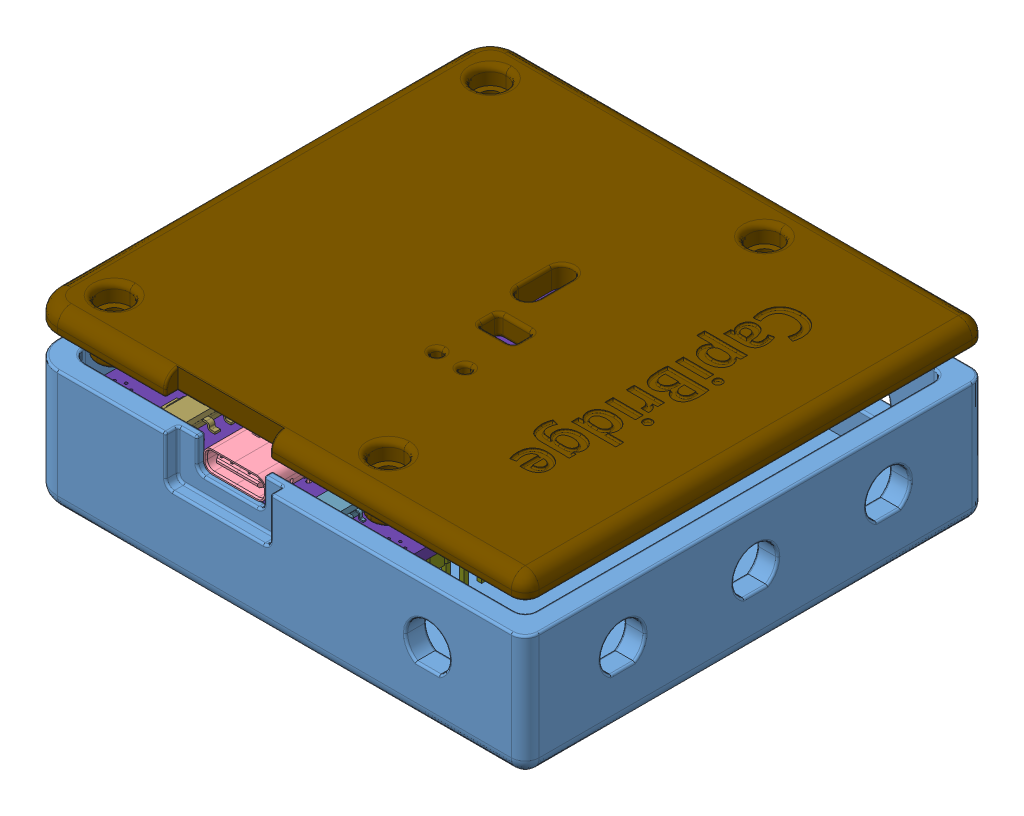
SolidWorks assembly Assem1, configuration Default. Lengths in mm.
Overall size (71 24.85 66.01).
68 component instances, 18 part files, 4 mates.
Components (placement in the parent):
- CapiBridge_Case.step-1: CapiBridge_Case.step [Default] at (49.0478 21.2808 49.0747) size (71 17.5 66.01)
- CapiBridge_PCB.step-1: CapiBridge_PCB.step [Default] at (23.5288 30.2808 76.9234) x (1 0 0) z (0 1 0) size (44.35 60.13 16.04)
  - C_0603_1608Metric.step-1: C_0603_1608Metric.step [Default] at (19.4987 21.1736 1.65) x (0 1 0) z (0 0 1) size (1.6 0.8 0.8)
    - C_0603_1608Metric-0.step-1: C_0603_1608Metric-0.step [Default] at origin size (1.6 0.8 0.8)
  - CP_EIA-3216-18_Kemet-A.step-1: CP_EIA-3216-18_Kemet-A.step [Default] at (11.2987 11.0736 1.65) size (3.2 1.6 1.8)
    - CP_EIA_3216_18_Kemet_A.step-1: CP_EIA_3216_18_Kemet_A.step [Default] at origin size (3.2 1.6 1.8)
  - USB_C_Receptacle_GCT_USB4105-xx-A_16P_TopMnt_Horizontal.step-1: USB_C_Receptacle_GCT_USB4105-xx-A_16P_TopMnt_Horizontal.step [Default] at (17.0087 0.9136 1.65) size (8.94 7.78 4.26)
    - USB_C_Receptacle_16P_TopMnt_Horizontal_GCT_USB4105-xx-A.step-1: USB_C_Receptacle_16P_TopMnt_Horizontal_GCT_USB4105-xx-A.step [Default] at origin size (8.94 7.78 4.26)
  - LED_0603_1608Metric.step-1: LED_0603_1608Metric.step [Default] at (25.3487 32.6736 1.65) size (1.6 0.8 1.1)
    - LED_0603_1608Metric-1.step-1: LED_0603_1608Metric-1.step [Default] at origin size (1.6 0.8 1.1)
  - YC164-FR-075K6L.step-1: YC164-FR-075K6L.step [Default] at (30.4987 33.3236 1.65) x (1 0 0) z (0 -1 0) size (1.6 0.7 3.2)
    - YC164-JR-0720KL.step-1: YC164-JR-0720KL.step [Default] at origin size (1.6 0.7 3.2)
  - CP_EIA-3528-21_Kemet-B.step-1: CP_EIA-3528-21_Kemet-B.step [Default] at (1.7987 9.5736 1.65) x (0 1 0) z (0 0 1) size (3.5 2.8 2.1)
    - CP_EIA_3528_21_Kemet_B.step-1: CP_EIA_3528_21_Kemet_B.step [Default] at origin size (3.5 2.8 2.1)
  - LED_0603_1608Metric.step-2: LED_0603_1608Metric.step [Default] at (25.3487 34.2236 1.65) size (1.6 0.8 1.1)
    - LED_0603_1608Metric-1.step-1: LED_0603_1608Metric-1.step [Default] at origin size (1.6 0.8 1.1)
  - ESP32-C3-WROOM-02U-N4.step-1: ESP32-C3-WROOM-02U-N4.step [Default] at (15.9527 35.9396 1.65) size (18 14.3 3.21)
    - 3D_PCB1_2022-06-18 v3.step-1: 3D_PCB1_2022-06-18 v3.step [Default] at origin size (18 14.3 3.21)
  - YC164-FR-075K6L.step-2: YC164-FR-075K6L.step [Default] at (20.3487 26.0736 1.65) x (0 -1 0) z (-1 0 0) size (1.6 0.7 3.2)
    - YC164-JR-0720KL.step-1: YC164-JR-0720KL.step [Default] at origin size (1.6 0.7 3.2)
  - C_0603_1608Metric.step-2: C_0603_1608Metric.step [Default] at (32.0987 6.8736 1.65) x (0 -1 0) z (0 0 1) size (1.6 0.8 0.8)
    - C_0603_1608Metric-0.step-1: C_0603_1608Metric-0.step [Default] at origin size (1.6 0.8 0.8)
  - SOT-363_SC-70-6.step-1: SOT-363_SC-70-6.step [Default] at (26.2487 11.2236 1.65) x (-1 0 0) z (0 0 1) size (2 2 1.05)
    - SOT_363_SC_70_6.step-1: SOT_363_SC_70_6.step [Default] at origin size (2 2 1.05)
  - RA-01H--3DModel-STEP-1.step-1: RA-01H--3DModel-STEP-1.step [Default] at (8.3787 22.6736 1.65) x (1 0 0) z (0 -1 0) size (16 3.4 17)
    - RA-01H.step-1: RA-01H.step [Default] at origin size (16 3.4 17)
  - C_0603_1608Metric.step-3: C_0603_1608Metric.step [Default] at (-1.8853 26.4736 1.65) x (0 1 0) z (0 0 1) size (1.6 0.8 0.8)
    - C_0603_1608Metric-0.step-1: C_0603_1608Metric-0.step [Default] at origin size (1.6 0.8 0.8)
  - SOT-143.step-1: SOT-143.step [Default] at (16.9851 8.7089 1.65) size (2.8 2.9 1.2)
    - SOT_143.step-1: SOT_143.step [Default] at origin size (2.8 2.9 1.2)
  - C_0603_1608Metric.step-4: C_0603_1608Metric.step [Default] at (-5.1336 49.1028 1.65) x (0 -1 0) z (0 0 1) size (1.6 0.8 0.8)
    - C_0603_1608Metric-0.step-1: C_0603_1608Metric-0.step [Default] at origin size (1.6 0.8 0.8)
  - C_0603_1608Metric.step-5: C_0603_1608Metric.step [Default] at (4.4987 9.0736 1.65) x (0 1 0) z (0 0 1) size (1.6 0.8 0.8)
    - C_0603_1608Metric-0.step-1: C_0603_1608Metric-0.step [Default] at origin size (1.6 0.8 0.8)
  - ESP32-C3-WROOM-02U-N4.step-2: ESP32-C3-WROOM-02U-N4.step [Default] at (-5.1973 35.9656 1.65) size (18 14.3 3.21)
    - 3D_PCB1_2022-06-18 v3.step-1: 3D_PCB1_2022-06-18 v3.step [Default] at origin size (18 14.3 3.21)
  - SOT-223.step-1: SOT-223.step [Default] at (5.3487 2.9736 1.65) x (-1 0 0) z (0 0 1) size (7 6.5 1.7)
    - SOT_223.step-1: SOT_223.step [Default] at origin size (7 6.5 1.7)
  - YC164-FR-075K6L.step-3: YC164-FR-075K6L.step [Default] at (30.4487 11.6736 1.65) x (1 0 0) z (0 -1 0) size (1.6 0.7 3.2)
    - YC164-JR-0720KL.step-1: YC164-JR-0720KL.step [Default] at origin size (1.6 0.7 3.2)
  - C_0603_1608Metric.step-6: C_0603_1608Metric.step [Default] at (21.0987 21.1736 1.65) x (0 1 0) z (0 0 1) size (1.6 0.8 0.8)
    - C_0603_1608Metric-0.step-1: C_0603_1608Metric-0.step [Default] at origin size (1.6 0.8 0.8)
  - LED_0603_1608Metric.step-3: LED_0603_1608Metric.step [Default] at (25.3487 35.8236 1.65) size (1.6 0.8 1.1)
    - LED_0603_1608Metric-1.step-1: LED_0603_1608Metric-1.step [Default] at origin size (1.6 0.8 1.1)
  - Selector Switch - MSS22D18.step-1: Selector Switch - MSS22D18.step [Default] at (28.2987 27.1236 6.9) x (1 0 0) z (0 -1 0) size (9.17 5.82 6.22)
    - Selector Switch - MSS22D18-2.step-1: Selector Switch - MSS22D18-2.step [Default] at origin size (9.17 5.82 6.22)
  - LED_0603_1608Metric.step-4: LED_0603_1608Metric.step [Default] at (20.4487 10.4236 1.65) x (0 1 0) z (0 0 1) size (1.6 0.8 1.1)
    - LED_0603_1608Metric-1.step-1: LED_0603_1608Metric-1.step [Default] at origin size (1.6 0.8 1.1)
  - SOIC-16_3.9x9.9mm_P1.27mm.step-1: SOIC-16_3.9x9.9mm_P1.27mm.step [Default] at (27.3987 4.3736 1.65) size (6 9.9 1.75)
    - SOIC_16_39x99mm_P127mm.step-1: SOIC_16_39x99mm_P127mm.step [Default] at origin size (6 9.9 1.75)
  - C_0603_1608Metric.step-7: C_0603_1608Metric.step [Default] at (16.0807 49.1515 1.65) x (0 1 0) z (0 0 1) size (1.6 0.8 0.8)
    - C_0603_1608Metric-0.step-1: C_0603_1608Metric-0.step [Default] at origin size (1.6 0.8 0.8)
  - LED_0603_1608Metric.step-5: LED_0603_1608Metric.step [Default] at (22.1487 10.4236 1.65) x (0 1 0) z (0 0 1) size (1.6 0.8 1.1)
    - LED_0603_1608Metric-1.step-1: LED_0603_1608Metric-1.step [Default] at origin size (1.6 0.8 1.1)
  - C_0603_1608Metric.step-8: C_0603_1608Metric.step [Default] at (7.3487 9.8736 1.65) x (-1 0 0) z (0 0 1) size (1.6 0.8 0.8)
    - C_0603_1608Metric-0.step-1: C_0603_1608Metric-0.step [Default] at origin size (1.6 0.8 0.8)
  - LED_0603_1608Metric.step-6: LED_0603_1608Metric.step [Default] at (25.3487 31.0736 1.65) size (1.6 0.8 1.1)
    - LED_0603_1608Metric-1.step-1: LED_0603_1608Metric-1.step [Default] at origin size (1.6 0.8 1.1)
  - D_SOD-123F.step-1: D_SOD-123F.step [Default] at (11.2987 8.6736 1.65) size (3.5 1.6 1.1)
    - D_SOD_123F.step-1: D_SOD_123F.step [Default] at origin size (3.5 1.6 1.1)
  - YC164-FR-075K6L.step-4: YC164-FR-075K6L.step [Default] at (20.2987 16.4736 1.65) x (0 1 0) z (1 0 0) size (1.6 0.7 3.2)
    - YC164-JR-0720KL.step-1: YC164-JR-0720KL.step [Default] at origin size (1.6 0.7 3.2)
  - PinHeader_1x12_P2.54mm_Vertical.step-1: PinHeader_1x12_P2.54mm_Vertical.step [Default] at (-4.62 5.9936 -0.05) x (1 0 0) z (0 0 -1) size (2.54 30.48 11.54)
    - PinHeader_1x12_P254mm_Vertical.step-1: PinHeader_1x12_P254mm_Vertical.step [Default] at origin size (2.54 30.48 11.54)
  - PinHeader_1x12_P2.54mm_Vertical.step-2: PinHeader_1x12_P2.54mm_Vertical.step [Default] at (36.02 5.9736 -0.05) x (1 0 0) z (0 0 -1) size (2.54 30.48 11.54)
    - PinHeader_1x12_P254mm_Vertical.step-1: PinHeader_1x12_P254mm_Vertical.step [Default] at origin size (2.54 30.48 11.54)
  - ESP-NOW_Gateway_PCB.step-1: ESP-NOW_Gateway_PCB.step [Default] at origin size (44.35 58.95 1.6)
- CapiBridge_Case_lit.step-1: CapiBridge_Case_lit.step [Default] at (49.0478 25.6289 49.0747) size (71 7.3 66)
Mates (geometry in assembly coordinates):
- Coincident1: coincident anti-aligned: plane of CapiBridge_Case.step-1 through (19.6278 30.2808 22.1497) normal (0 1 0); plane of CapiBridge_PCB.step-1/ESP-NOW_Gateway_PCB.step-1 through (39.2538 30.2808 49.0247) normal (0 -1 0)
- Concentric2: concentric anti-aligned: cylinder of CapiBridge_Case.step-1 through (58.8788 17.0381 75.9997) axis (0 1 0) radius 1.5; cylinder of CapiBridge_PCB.step-1/ESP-NOW_Gateway_PCB.step-1 through (58.8788 30.2358 75.9997) axis (0 -1 0) radius 1.1
- Coincident6: coincident aligned: plane of CapiBridge_Case.step-1 through (13.5478 36.2808 16.0747) normal (-1 0 0); plane of CapiBridge_Case_lit.step-1 through (13.5478 40.6289 16.0747) normal (-1 0 0)
- Coincident7: coincident aligned: plane of CapiBridge_Case.step-1 through (13.5478 36.2808 16.0747) normal (0 0 -1); plane of CapiBridge_Case_lit.step-1 through (13.5478 40.6289 16.0747) normal (0 0 -1)
